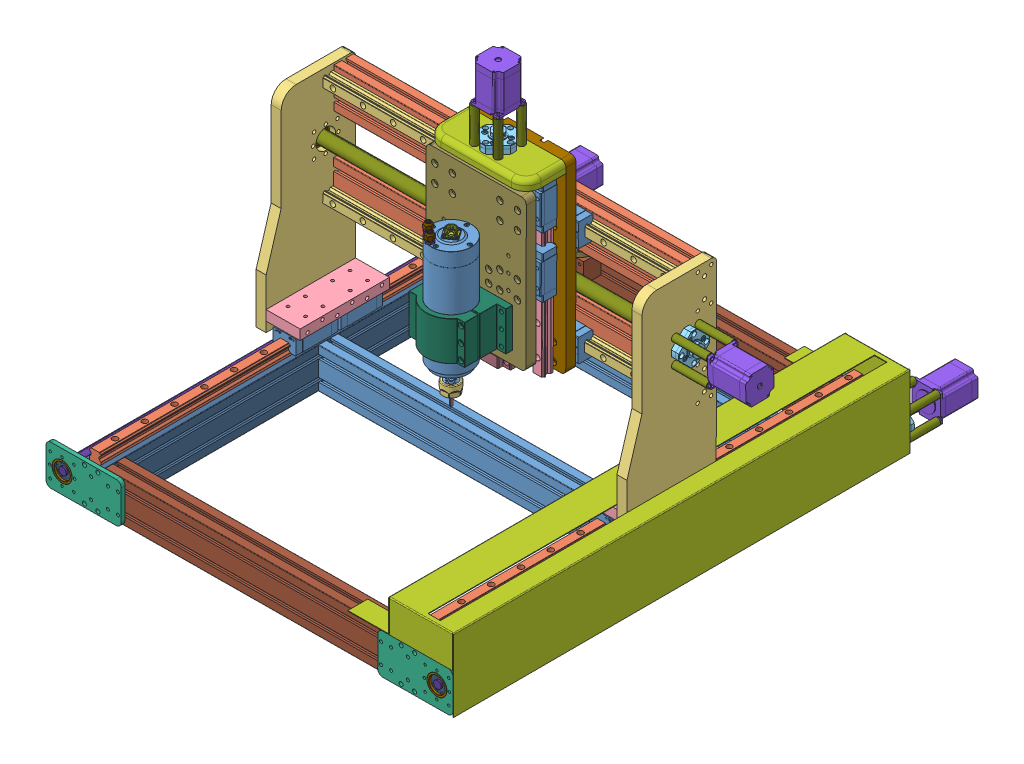
SolidWorks assembly cnc machine, configuration 默认. Lengths in mm. (continued)
Mates (geometry in assembly coordinates): (continued)
- Concentric138: concentric: cylinder of 57BYG250C-3 through (786.0531 509.1221 -21.2847) axis (-0.004945 -0.003582 -0.999981) radius 4; cylinder of FK_15Yes_FS-3/_FK_15collar_4-1 through (786.4013 509.3743 49.1139) axis (-0.004945 -0.003582 -0.999981) radius 7.5
- Parallel7: parallel: plane of back-2 through (386.56 716.0099 462.5509) normal (-0.999986 -0.00209 0.004953); plane of sfu25unit-4/slidernutSLDPRT-1 through (466.0897 826.0042 413.7627) normal (-0.999986 -0.00209 0.004953)
- Parallel8: parallel: plane of back-2 through (486.1687 901.2173 461.3948) normal (-0.004945 -0.003582 -0.999981); plane of sfu25unit-4/slidernutSLDPRT-1 through (506.0891 826.0878 413.5646) normal (-0.004945 -0.003582 -0.999981)
- Concentric178: concentric: cylinder of top plate-1 through (486.0978 1066.4165 516.8045) axis (-0.002108 0.999991 -0.003572) radius 20; cylinder of sfu25unit-5/SFU2505-1 through (486.4038 921.2727 517.3229) axis (-0.002108 0.999991 -0.003572) radius 12.5
- Parallel10: parallel: plane of back-2 through (486.2676 901.289 481.3945) normal (0.004945 0.003582 0.999981); plane of sfu25unit-5/slidernutSLDPRT-1 through (453.544 911.2898 541.5216) normal (0.004945 0.003582 0.999981)
- Concentric181: concentric: cylinder of linerrailHGGR25400-2 through (763.4076 958.1784 441.5619) axis (-0.999986 -0.00209 0.004953) radius 2.43; cylinder of HGH25CA-6 through (398.9607 957.4167 443.367) axis (0.999986 0.00209 -0.004953) radius 2.43
- Coincident354: coincident: plane of back-2 through (386.56 716.0099 462.5509) normal (-0.999986 -0.00209 0.004953); plane of motorseat-2 through (386.3277 1061.2201 561.3173) normal (-0.999986 -0.00209 0.004953)
- Coincident355: coincident: plane of back-2 through (586.5572 716.4279 461.5603) normal (0.999986 0.00209 -0.004953); plane of motorseat-2 through (586.3248 1061.6381 560.3268) normal (0.999986 0.00209 -0.004953)
- Concentric183: concentric: cylinder of linerrailHGGR25300-1 through (421.2087 981.2312 503.4303) axis (0.004945 0.003582 0.999981) radius 5.5; cylinder of back-2 through (421.001 981.0808 461.4311) axis (-0.004945 -0.003582 -0.999981) radius 2.5
- Concentric185: concentric: cylinder of HGH25CA-11 through (438.94 913.6879 521.5849) axis (0.004945 0.003582 0.999981) radius 3; cylinder of motorseat-2 through (439.1378 913.8311 561.5841) axis (0.004945 0.003582 0.999981) radius 6.5
- Concentric186: concentric: circle of top plate-1; circle of sfu25unit-5/SFU2505-1
- Concentric187: concentric: cylinder of top plate-1 through (486.0978 1066.4165 516.8045) axis (-0.002108 0.999991 -0.003572) radius 20; cylinder of sfu25unit-5/SFU2505-1 through (486.4038 921.2727 517.3229) axis (-0.002108 0.999991 -0.003572) radius 12.5
- Concentric188: concentric: cylinder of linerrailHGGR25300-1 through (432.4857 1061.2535 502.8303) axis (0.002108 -0.999991 0.003572) radius 2.43; cylinder of HGH25CA-12 through (432.5197 1045.1087 502.888) axis (0.002108 -0.999991 0.003572) radius 2.43
- Concentric189: concentric: cylinder of linerrailHGGR25300-1 through (409.5919 1061.2067 502.9437) axis (0.002108 -0.999991 0.003572) radius 2.43; cylinder of HGH25CA-12 through (409.6259 1045.0608 503.0014) axis (0.002108 -0.999991 0.003572) radius 2.43
- Concentric190: concentric: cylinder of HGH25CA-12 through (403.6876 1033.6137 521.3296) axis (0.004945 0.003582 0.999981) radius 3; cylinder of motorseat-2 through (403.8854 1033.757 561.3289) axis (0.004945 0.003582 0.999981) radius 6.5
- Coincident357: coincident: plane of HGH25CA-12 through (407.6633 1045.1219 521.2687) normal (0.004945 0.003582 0.999981); plane of 10mmwasher-1 through (422.2242 1016.1525 521.3005) normal (-0.004945 -0.003582 -0.999981)
- Coincident358: coincident: plane of HGH25CA-12 through (421.1963 987.0862 503.4094) normal (0.002108 -0.999991 0.003572); plane of 10mmwasher-1 through (447.285 987.205 521.2802) normal (0.002108 -0.999991 0.003572)
- Coincident359: coincident: plane of 10mmwasher-1 through (422.3231 1016.2241 541.3001) normal (0.004945 0.003582 0.999981); plane of motorseat-2 through (486.5435 911.3588 541.3582) normal (-0.004945 -0.003582 -0.999981)
- Concentric192: concentric: cylinder of sfu25unit-5/slidernutSLDPRT-1 through (461.5607 903.3066 541.5105) axis (0.004945 0.003582 0.999981) radius 2.5; cylinder of motorseat-2 through (461.6596 903.3782 561.5102) axis (0.004945 0.003582 0.999981) radius 3.3
- Coincident360: coincident: plane of 80_2-1 through (486.7394 865.4308 561.5221) normal (-0.004945 -0.003582 -0.999981); plane of motorseat-2 through (486.6424 911.4304 561.3578) normal (0.004945 0.003582 0.999981)
- Concentric193: concentric: cylinder of top plate-1 through (509.7433 1086.55 540.1873) axis (-0.002108 0.999991 -0.003572) radius 2.5; cylinder of motor conectors-4/motor connector-2 through (509.7433 1086.55 540.1873) axis (-0.002108 0.999991 -0.003572) radius 7
- Coincident361: coincident: plane of 57BYG250C-1 through (485.9081 1156.4157 516.483) normal (0.002108 -0.999991 0.003572); plane of motor conectors-4/motor connector-1 through (462.4536 1156.4509 540.1694) normal (-0.002108 0.999991 -0.003572)
- Concentric196: concentric: cylinder of 80_2-1 through (551.4531 796.6164 575.4488) axis (0.004945 0.003582 0.999981) radius 4; cylinder of motorseat-2 through (551.3839 796.5662 561.4491) axis (0.004945 0.003582 0.999981) radius 3.4
- Coincident363: coincident: plane of HGH25CA-12 through (397.156 1045.0946 519.8208) normal (-0.999986 -0.00209 0.004953); plane of 10mmwasher-1 through (397.1635 1045.1 521.3207) normal (-0.999986 -0.00209 0.004953)
- Concentric200: concentric: cylinder of back-2 through (513.636 726.3469 481.8858) axis (0.004945 0.003582 0.999981) radius 2.5; cylinder of BF_15-1/_BF_15_Part1_2-1 through (513.6756 726.3756 489.8856) axis (0.004945 0.003582 0.999981) radius 3.3
- Concentric201: concentric: cylinder of back-2 through (459.6368 726.234 482.1532) axis (0.004945 0.003582 0.999981) radius 2.5; cylinder of BF_15-1/_BF_15_Part1_2-1 through (459.6764 726.2627 490.1531) axis (0.004945 0.003582 0.999981) radius 5.5
- Coincident373: coincident: plane of BF_15-1/_BF_15_Part1_2-1 through (452.8554 736.2484 490.151) normal (-0.004945 -0.003582 -0.999981); plane of 8mmwasher-1 through (486.676 726.2625 490.0196) normal (0.004945 0.003582 0.999981)
- Concentric202: concentric: cylinder of BF_15-1/_BF_15_Part1_2-1 through (459.6764 726.2627 490.1531) axis (0.004945 0.003582 0.999981) radius 3.3; cylinder of 8mmwasher-1 through (459.6764 726.2627 490.1531) axis (-0.004945 -0.003582 -0.999981) radius 3
- Coincident374: coincident: plane of back-2 through (486.2676 901.289 481.3945) normal (0.004945 0.003582 0.999981); plane of 8mmwasher-1 through (486.6365 726.2338 482.0197) normal (-0.004945 -0.003582 -0.999981)
- Concentric203: concentric: cylinder of sfu25unit-5/SFU2505-1 through (486.4038 921.2727 517.3229) axis (-0.002108 0.999991 -0.003572) radius 12.5; cylinder of BF_15-1/_BF_15_Part2_4-1 through (486.7091 776.419 517.8402) axis (0.002108 -0.999991 0.003572) radius 7.5
- Concentric204: concentric: cylinder of FK_15Yes_FS-1/_FK_15_FS_1_2-1 through (800.6126 846.789 436.0343) axis (0.999986 0.00209 -0.004953) radius 6.9585; cylinder of screw2-1 through (34.6237 845.1881 439.8282) axis (-0.999986 -0.00209 0.004953) radius 12.5
- Concentric205: concentric: cylinder of FK_15Yes_FS-3/_FK_15collar_4-1 through (786.4013 509.3743 49.1139) axis (-0.004945 -0.003582 -0.999981) radius 7.5; cylinder of screw2 - right left-1 through (790.8224 512.5765 943.0973) axis (0.004945 0.003582 0.999981) radius 12.5
- Coincident376: coincident: plane of FF_15-2/_FF_15_Part2_4-1 through (789.6322 497.0249 931.1586) normal (-0.004945 -0.003582 -0.999981); plane of screw2 - right left-1 through (784.5914 523.4037 931.0891) normal (0.004945 0.003582 0.999981)
- Concentric206: concentric: cylinder of FK_15Yes_FS-2/_FK_15collar_4-1 through (38.4121 507.8109 52.8186) axis (-0.004945 -0.003582 -0.999981) radius 7.5; cylinder of screw2 - right left-2 through (42.8332 511.0132 946.8029) axis (0.004945 0.003582 0.999981) radius 12.5
- Concentric207: concentric: cylinder of FK_15Yes_FS-4/_FK_15collar_4-1 through (486.0999 1065.4165 516.8081) axis (-0.002108 0.999991 -0.003572) radius 7.5; cylinder of screw2 top-1 through (486.8387 714.9195 518.0599) axis (0.002108 -0.999991 0.003572) radius 12.5
- Concentric208: concentric: cylinder of 80_2-1 through (422.3285 856.3462 575.8734) axis (0.004945 0.003582 0.999981) radius 4; cylinder of motorseat-2 through (422.2593 856.2961 561.8737) axis (0.004945 0.003582 0.999981) radius 3.4
- Distance2: distance = 10 mm: plane of 80_2.2Kw-2/Шпиндель Ø80_2.2Kw.stp-1/D880_2.2Kw.stp-1 through (467.4776 751.469 583.8543) normal (0.002108 -0.999991 0.003572); plane of motorseat-2 through (386.96 761.2227 562.3888) normal (0.002108 -0.999991 0.003572)
- Concentric210: concentric: cylinder of linerrailHGGR25-1 through (99.5791 572.3208 719.2975) axis (-0.002108 0.999991 -0.003572) radius 5.5; cylinder of nuts-4 through (100.2578 250.3236 720.4475) axis (-0.002108 0.999991 -0.003572) radius 2.4112
- Concentric211: concentric: cylinder of linerrailHGGR25-2 through (716.7608 570.9245 36.2366) axis (0.004945 0.003582 0.999981) radius 2.43; cylinder of HGH25CA-4 through (718.9723 572.5263 483.4213) axis (0.004945 0.003582 0.999981) radius 2.43
- Coincident409: coincident: plane of bottom-1/EF4080-t5-900-2 through (712.7555 528.2383 936.4271) normal (-0.999986 -0.00209 0.004953); plane of EF4080-t5 -592-1 through (709.0064 544.7019 186.43) normal (0.999986 0.00209 -0.004953)
- Coincident410: coincident: plane of bottom-1/EF4080-t5-900-2 through (712.7046 552.3881 936.3409) normal (-0.002108 0.999991 -0.003572); plane of EF4080-t5 -592-1 through (708.897 549.6302 166.4125) normal (-0.002108 0.999991 -0.003572)
- Concentric225: concentric: cylinder of sfu25unit-3/SFU2505-1 through (788.3952 510.8185 452.2985) axis (0.004945 0.003582 0.999981) radius 12.5; cylinder of screw2 - right left-1 through (790.8224 512.5765 943.0973) axis (0.004945 0.003582 0.999981) radius 12.5
- Distance5: limit distance = 134.855 mm: plane of BF_15-1/_BF_15_Part1_2-1 through (486.7934 736.4193 517.9831) normal (-0.002108 0.999991 -0.003572); plane of sfu25unit-5/slidernutSLDPRT-1 through (506.3902 871.229 493.4029) normal (0.002108 -0.999991 0.003572)
- Concentric241: concentric: cylinder of FF_15-1/_FF_15_Part2_4-1 through (43.0434 511.1654 989.3021) axis (-0.004945 -0.003582 -0.999981) radius 7.5; cylinder of screw2 - right left-2 through (42.8332 511.0132 946.8029) axis (0.004945 0.003582 0.999981) radius 12.5
- Coincident456: coincident: plane of FK_15Yes_FS-1/_FK_15collar_4-1 through (762.6288 839.2096 436.2225) normal (-0.999986 -0.00209 0.004953); plane of screw2-1 through (762.6356 839.3453 437.6426) normal (0.999986 0.00209 -0.004953)
- Coincident457: coincident: plane of FF_15-1/_FF_15_Part2_4-1 through (42.6559 495.4208 934.8594) normal (-0.004945 -0.003582 -0.999981); plane of screw2 - right left-2 through (38.9401 499.0728 934.8647) normal (0.004945 0.003582 0.999981)
- Coincident458: coincident: plane of 57BYG250C-2 through (37.9621 507.485 -38.1797) normal (0.004945 0.003582 0.999981); plane of motor conectors-5/motor connector-1 through (14.3427 531.0055 -38.1471) normal (-0.004945 -0.003582 -0.999981)
- Coincident459: coincident: plane of BF_15-1/_BF_15_Part2_4-1 through (486.7664 730.8914 510.2029) normal (-0.002108 0.999991 -0.003572); plane of screw2 top-1 through (474.3221 730.8954 518.657) normal (0.002108 -0.999991 0.003572)
- Coincident462: coincident: plane of linerrailHGGR25-1 through (112.2132 551.133 939.315) normal (0.002108 -0.999991 0.003572); plane of bottom-1/EF4080-t5-900-1 through (120.7131 551.1508 939.2729) normal (-0.002108 0.999991 -0.003572)
- Coincident463: coincident: plane of nuts-4 through (93.4719 547.0939 939.4222) normal (-0.002108 0.999991 -0.003572); plane of bottom-1/EF4080-t5-900-1 through (96.5719 547.1004 939.4068) normal (0.002108 -0.999991 0.003572)
- Coincident464: coincident: plane of nuts-4 through (96.5719 547.1004 939.4068) normal (-0.999986 -0.00209 0.004953); plane of bottom-1/EF4080-t5-900-1 through (96.5635 551.1003 939.3925) normal (0.999986 0.00209 -0.004953)
- Concentric252: concentric: cylinder of linerrailHGGR25-1 through (99.8758 572.5357 779.2964) axis (-0.002108 0.999991 -0.003572) radius 5.5; cylinder of nuts-4 through (100.5545 250.5385 780.4464) axis (-0.002108 0.999991 -0.003572) radius 2.4112
- Coincident469: coincident: plane of side right - final-5 through (64.7984 569.6809 560.668) normal (0.004945 0.003582 0.999981); plane of bottom-2 through (132.7131 609.8227 560.1884) normal (0.004945 0.003582 0.999981)
- Coincident473: coincident: plane of HGH25CA-2 through (120.4444 589.2114 396.3198) normal (-0.002108 0.999991 -0.003572); plane of bottom-2 through (98.3107 589.4294 470.4299) normal (0.002108 -0.999991 0.003572)
- Coincident477: coincident: plane of sfu25unit-1/slidernutSLDPRT-1 through (64.0888 542.1259 405.7674) normal (0.999986 0.00209 -0.004953); plane of conn12-1 through (63.8661 589.036 380.6) normal (-0.999986 -0.00209 0.004953)
- Concentric257: concentric: cylinder of sfu25unit-1/SFU2505-1 through (40.1093 509.0402 396.0043) axis (-0.004945 -0.003582 -0.999981) radius 12.5; cylinder of FK_15Yes_FS-2/_FK_15_FS_1_2-1 through (38.3923 507.7966 48.8187) axis (-0.004945 -0.003582 -0.999981) radius 20
- Concentric259: concentric: cylinder of 57BYG250C-2 through (14.3427 531.0055 -38.1471) axis (-0.004945 -0.003582 -0.999981) radius 2.55; cylinder of motor conectors-5/motor connector-1 through (14.3427 531.0055 -38.1471) axis (0.004945 0.003582 0.999981) radius 3
- Concentric260: concentric: cylinder of FK_15Yes_FS-2/_FK_15_FS_1_2-1 through (38.3923 507.7966 48.8187) axis (-0.004945 -0.003582 -0.999981) radius 20; cylinder of mot1-1 through (38.3082 507.7357 31.819) axis (0.004945 0.003582 0.999981) radius 20
- Concentric261: concentric: cylinder of bottom-1/EF4080-t5-900-1 through (87.2273 544.5808 939.462) axis (-0.004945 -0.003582 -0.999981) radius 4; cylinder of mot1-1 through (82.7765 541.3571 39.4788) axis (0.004945 0.003582 0.999981) radius 4
- Concentric262: concentric: cylinder of bottom-1/EF4080-t5-900-1 through (114.2269 544.6373 939.3283) axis (-0.004945 -0.003582 -0.999981) radius 4; circle of mot1-1
- Coincident483: coincident: plane of bottom-1/EF4080-t5-900-1 through (96.4207 472.8859 39.6566) normal (-0.004945 -0.003582 -0.999981); plane of mot1-1 through (81.3472 507.8542 39.6059) normal (0.004945 0.003582 0.999981)
- Coincident484: coincident: plane of FK_15Yes_FS-2/_FK_15_FS_1_2-1 through (38.2429 538.7354 31.7083) normal (0.004945 0.003582 0.999981); plane of mot1-1 through (81.3076 507.8256 31.6061) normal (-0.004945 -0.003582 -0.999981)
- Concentric263: concentric: cylinder of FK_15Yes_FS-2/_FK_15_FS_1_2-1 through (38.2555 532.7355 31.7297) axis (-0.004945 -0.003582 -0.999981) radius 4.75; cylinder of mot1-1 through (38.2951 532.7641 39.7296) axis (0.004945 0.003582 0.999981) radius 2.5
- Concentric264: concentric: cylinder of motor conectors-5/motor connector-1 through (14.3427 531.0055 -38.1471) axis (0.004945 0.003582 0.999981) radius 7; cylinder of mot1-1 through (14.7285 531.2849 39.8514) axis (0.004945 0.003582 0.999981) radius 2.5
- Parallel11: parallel: plane of 57BYG250C-2 through (21.3864 535.4216 -102.199) normal (-0.002108 0.999991 -0.003572); plane of mot1-1 through (6.2639 547.6971 39.8345) normal (-0.002108 0.999991 -0.003572)
- Coincident485: coincident: plane of motor conectors-5/motor connector-1 through (14.6889 531.2562 31.8516) normal (0.004945 0.003582 0.999981); plane of mot1-1 through (81.3076 507.8256 31.6061) normal (-0.004945 -0.003582 -0.999981)
- Coincident486: coincident: plane of linerrailHGGR25-1 through (96.2163 569.8851 39.3102) normal (-0.004945 -0.003582 -0.999981); plane of bottom-1/EF4080-t5 -540-2 through (708.2538 549.1643 36.3576) normal (-0.004945 -0.003582 -0.999981)
- Concentric266: concentric: cylinder of linerrailHGGR25-2 through (716.7608 570.9245 36.2366) axis (0.004945 0.003582 0.999981) radius 2.43; cylinder of HGH25CA-3 through (718.5272 572.204 393.423) axis (0.004945 0.003582 0.999981) radius 2.43
- Coincident487: coincident: plane of linerrailHGGR25-2 through (744.2041 552.4539 936.1848) normal (0.002108 -0.999991 0.003572); plane of bottom-1/EF4080-t5-900-2 through (752.704 552.4717 936.1427) normal (-0.002108 0.999991 -0.003572)
- Concentric268: concentric: cylinder of EF4080-t5 -800-1 through (763.2626 960.1301 413.3126) axis (-0.999986 -0.00209 0.004953) radius 4; cylinder of side right - final-5 through (63.2728 958.6671 416.7796) axis (0.999986 0.00209 -0.004953) radius 3.4
- Concentric269: concentric: cylinder of EF4080-t5 -800-1 through (763.4039 893.1307 413.5519) axis (-0.999986 -0.00209 0.004953) radius 4; cylinder of side right - final-5 through (63.414 891.6677 417.0189) axis (0.999986 0.00209 -0.004953) radius 3.4
- Coincident488: coincident: plane of EF4080-t5 -800-1 through (63.3504 890.1194 403.5245) normal (-0.999986 -0.00209 0.004953); plane of side right - final-5 through (63.7314 789.1454 437.8425) normal (0.999986 0.00209 -0.004953)
- Concentric271: concentric: cylinder of EF4080-t5 -800-2 through (763.5999 800.1315 413.8841) axis (-0.999986 -0.00209 0.004953) radius 4; cylinder of side right - final-5 through (63.61 798.6685 417.351) axis (0.999986 0.00209 -0.004953) radius 3.4
- Concentric272: concentric: cylinder of EF4080-t5 -800-1 through (763.1291 960.0334 386.3131) axis (-0.999986 -0.00209 0.004953) radius 4; cylinder of side right - final-6 through (783.1288 960.0752 386.2141) axis (0.999986 0.00209 -0.004953) radius 3.4
- Coincident489: coincident: plane of EF4080-t5 -800-2 through (763.6775 731.5837 400.629) normal (0.999986 0.00209 -0.004953); plane of side right - final-6 through (763.7213 790.6084 434.3756) normal (-0.999986 -0.00209 0.004953)
- Concentric273: concentric: cylinder of EF4080-t5 -800-2 through (763.6076 733.0354 387.1239) axis (-0.999986 -0.00209 0.004953) radius 4; cylinder of side right - final-6 through (783.6073 733.0772 387.0248) axis (0.999986 0.00209 -0.004953) radius 3.4
- Coincident490: coincident: plane of EF4080-t5 -800-2 through (63.6876 730.1207 404.0959) normal (-0.999986 -0.00209 0.004953); plane of side right - final-5 through (63.7314 789.1454 437.8425) normal (0.999986 0.00209 -0.004953)
- Coincident493: coincident: plane of nuts-3 through (737.7867 546.869 496.2284) normal (-0.002108 0.999991 -0.003572); plane of bottom-1/EF4080-t5-900-2 through (736.8626 548.4386 936.2355) normal (0.002108 -0.999991 0.003572)
- Coincident494: coincident: plane of nuts-3 through (726.3784 550.8452 496.2706) normal (-0.999986 -0.00209 0.004953); plane of bottom-1/EF4080-t5-900-2 through (728.5543 552.4212 936.2624) normal (0.999986 0.00209 -0.004953)
- Concentric276: concentric: cylinder of linerrailHGGR25-2 through (730.6798 572.9969 536.1707) axis (-0.002108 0.999991 -0.003572) radius 5.5; cylinder of nuts-3 through (731.3585 250.9997 537.3207) axis (-0.002108 0.999991 -0.003572) radius 2.4112
- Concentric277: concentric: cylinder of linerrailHGGR25-2 through (731.2732 573.4268 656.1684) axis (-0.002108 0.999991 -0.003572) radius 3.5; cylinder of nuts-3 through (731.9519 251.4295 657.3185) axis (-0.002108 0.999991 -0.003572) radius 2.4112
- Concentric278: concentric: cylinder of HGH25CA-1 through (116.1195 589.6899 532.8421) axis (-0.002108 0.999991 -0.003572) radius 3; cylinder of bottom-2 through (116.0774 609.6897 532.7706) axis (-0.002108 0.999991 -0.003572) radius 3
- Coincident496: coincident: plane of side right - final-5 through (63.7314 789.1454 437.8425) normal (0.999986 0.00209 -0.004953); plane of bottom-2 through (64.7141 609.6806 560.5252) normal (-0.999986 -0.00209 0.004953)
- Concentric279: concentric: cylinder of side right - final-5 through (64.6694 595.6269 545.5755) axis (0.999986 0.00209 -0.004953) radius 4; cylinder of bottom-2 through (64.6694 595.6269 545.5755) axis (-0.999986 -0.00209 0.004953) radius 3.4
- Concentric280: concentric: cylinder of side right - final-5 through (63.9529 583.0898 395.6211) axis (0.999986 0.00209 -0.004953) radius 4; cylinder of conn12-1 through (63.9529 583.0898 395.6211) axis (-0.999986 -0.00209 0.004953) radius 3.4
- Concentric281: concentric: cylinder of side right - final-5 through (64.2497 583.3047 455.62) axis (0.999986 0.00209 -0.004953) radius 4; cylinder of conn12-1 through (64.2497 583.3047 455.62) axis (-0.999986 -0.00209 0.004953) radius 3.4
- Concentric282: concentric: cylinder of HGH25CA-2 through (80.5019 589.169 408.0177) axis (-0.002108 0.999991 -0.003572) radius 3; cylinder of bottom-2 through (80.4597 609.1688 407.9463) axis (-0.002108 0.999991 -0.003572) radius 3
- Coincident498: coincident: plane of linerrailHGGR25400-3 through (763.8536 746.7341 442.5746) normal (0.999986 0.00209 -0.004953); plane of side right - final-6 through (763.7213 790.6084 434.3756) normal (-0.999986 -0.00209 0.004953)
- Concentric285: concentric: cylinder of side right - final-6 through (783.9004 604.5944 391.9837) axis (0.999986 0.00209 -0.004953) radius 4; cylinder of bottom-3 through (695.9017 604.4105 392.4195) axis (-0.999986 -0.00209 0.004953) radius 3.4
- Coincident502: coincident: plane of side right - final-6 through (763.7213 790.6084 434.3756) normal (-0.999986 -0.00209 0.004953); plane of bottom-3 through (763.856 590.499 377.133) normal (0.999986 0.00209 -0.004953)
- Concentric286: concentric: cylinder of side right - final-6 through (784.659 597.1318 542.0094) axis (0.999986 0.00209 -0.004953) radius 4; cylinder of bottom-3 through (696.6603 596.9478 542.4453) axis (-0.999986 -0.00209 0.004953) radius 3.4
- Coincident503: coincident: plane of side right - final-6 through (763.7213 790.6084 434.3756) normal (-0.999986 -0.00209 0.004953); plane of conn12-2 through (764.3011 590.8214 467.1313) normal (0.999986 0.00209 -0.004953)
- Concentric288: concentric: cylinder of side right - final-6 through (783.9425 584.5946 392.0551) axis (0.999986 0.00209 -0.004953) radius 4; cylinder of conn12-2 through (763.9428 584.5528 392.1542) axis (0.999986 0.00209 -0.004953) radius 3.4
- Concentric289: concentric: cylinder of side right - final-6 through (784.2393 584.8095 452.054) axis (0.999986 0.00209 -0.004953) radius 4; cylinder of conn12-2 through (764.2396 584.7677 452.153) axis (0.999986 0.00209 -0.004953) radius 3.4
- Concentric290: concentric: cylinder of sfu25unit-3/slidernutSLDPRT-1 through (764.2538 535.7036 434.3284) axis (-0.999986 -0.00209 0.004953) radius 2.5; cylinder of conn12-2 through (764.2538 535.7036 434.3284) axis (0.999986 0.00209 -0.004953) radius 6.5
- Concentric291: concentric: cylinder of sfu25unit-3/slidernutSLDPRT-1 through (764.1351 535.6177 410.3288) axis (-0.999986 -0.00209 0.004953) radius 2.5; cylinder of conn12-2 through (764.1351 535.6177 410.3288) axis (0.999986 0.00209 -0.004953) radius 6.5
- Coincident504: coincident: plane of sfu25unit-3/slidernutSLDPRT-1 through (764.2765 543.7322 442.2997) normal (-0.999986 -0.00209 0.004953); plane of conn12-2 through (764.3011 590.8214 467.1313) normal (0.999986 0.00209 -0.004953)
- Concentric292: concentric: cylinder of bottom-1/EF4080-t5-900-2 through (719.2182 545.9017 936.3319) axis (-0.004945 -0.003582 -0.999981) radius 4; cylinder of mot1-2 through (714.7674 542.678 36.3487) axis (0.004945 0.003582 0.999981) radius 4
- Coincident505: coincident: plane of bottom-1/EF4080-t5-900-2 through (728.2641 544.2062 36.2764) normal (-0.004945 -0.003582 -0.999981); plane of mot1-2 through (743.3376 509.2378 36.3272) normal (0.004945 0.003582 0.999981)
- Concentric293: concentric: cylinder of FK_15Yes_FS-3/_FK_15_FS_1_2-1 through (786.3815 509.3599 45.114) axis (-0.004945 -0.003582 -0.999981) radius 20; cylinder of mot1-2 through (786.2974 509.2991 28.1143) axis (0.004945 0.003582 0.999981) radius 20
- Coincident506: coincident: plane of FK_15Yes_FS-3/_FK_15_FS_1_2-1 through (786.2298 540.2988 28.0036) normal (0.004945 0.003582 0.999981); plane of mot1-2 through (743.298 509.2092 28.3273) normal (-0.004945 -0.003582 -0.999981)
- Concentric294: concentric: cylinder of HGH25CA-4 through (713.1109 590.9376 529.8852) axis (-0.002108 0.999991 -0.003572) radius 3; cylinder of bottom-3 through (713.1109 590.9376 529.8852) axis (0.002108 -0.999991 0.003572) radius 3
- Concentric295: concentric: cylinder of HGH25CA-3 through (712.4927 590.4899 404.8876) axis (-0.002108 0.999991 -0.003572) radius 3; cylinder of bottom-3 through (712.4927 590.4899 404.8876) axis (0.002108 -0.999991 0.003572) radius 3
- Coincident507: coincident: plane of linerrailHGGR25-2 through (728.2071 571.206 36.18) normal (-0.004945 -0.003582 -0.999981); plane of mot1-2 through (743.3376 509.2378 36.3272) normal (0.004945 0.003582 0.999981)
- Coincident508: coincident: plane of motor conectors-1/motor connector-1 through (760.9197 533.2118 28.1542) normal (0.004945 0.003582 0.999981); plane of mot1-2 through (743.298 509.2092 28.3273) normal (-0.004945 -0.003582 -0.999981)
- Coincident509: coincident: plane of bottom-1/EF4080-t5-900-1 through (100.8715 476.1097 939.6398) normal (0.004945 0.003582 0.999981); plane of mot1-4 through (85.7979 511.078 939.5891) normal (-0.004945 -0.003582 -0.999981)
- Concentric296: concentric: cylinder of bottom-1/EF4080-t5-900-1 through (114.2269 544.6373 939.3283) axis (-0.004945 -0.003582 -0.999981) radius 4; cylinder of mot1-4 through (114.2665 544.6659 947.3282) axis (0.004945 0.003582 0.999981) radius 4
- Concentric297: concentric: circle of sfu25unit-1/slidernutSLDPRT-1; cylinder of conn12-1 through (64.2639 534.2406 437.7953) axis (-0.999986 -0.00209 0.004953) radius 6.5
- Coincident510: coincident: plane of FF_15-2/_FF_15Part1_2-1 through (793.0421 543.4692 935.9755) normal (0.004945 0.003582 0.999981); plane of mot1-3 through (747.7884 512.4616 936.3104) normal (-0.004945 -0.003582 -0.999981)
- Concentric298: concentric: cylinder of FF_15-2/_FF_15Part1_2-1 through (790.5405 512.3724 886.0983) axis (0.004945 0.003582 0.999981) radius 20; cylinder of mot1-3 through (790.7877 512.5515 936.0974) axis (0.004945 0.003582 0.999981) radius 20
- Concentric299: concentric: cylinder of FF_15-2/_FF_15_Part2_4-1 through (791.0325 512.7288 985.5965) axis (-0.004945 -0.003582 -0.999981) radius 7.5; cylinder of screw2 - right left-1 through (790.8224 512.5765 943.0973) axis (0.004945 0.003582 0.999981) radius 12.5
- Coincident511: coincident: plane of bottom-1/EF4080-t5-900-2 through (732.7148 547.4299 936.2597) normal (0.004945 0.003582 0.999981); plane of mot1-3 through (747.7884 512.4616 936.3104) normal (-0.004945 -0.003582 -0.999981)
- Concentric300: concentric: cylinder of bottom-1/EF4080-t5-900-2 through (719.2182 545.9017 936.3319) axis (-0.004945 -0.003582 -0.999981) radius 4; cylinder of mot1-3 through (719.2577 545.9304 944.3317) axis (0.004945 0.003582 0.999981) radius 4
- Coincident512: coincident: plane of linerrailHGGR25400-2 through (63.3576 933.6906 423.3687) normal (-0.004945 -0.003582 -0.999981); plane of EF4080-t5 -800-1 through (763.3988 910.8038 419.9887) normal (0.004945 0.003582 0.999981)
- Concentric304: concentric: cylinder of screw2-1 through (34.6237 845.1881 439.8282) axis (-0.999986 -0.00209 0.004953) radius 12.5; cylinder of side right - final-6 through (763.6131 846.7117 436.2176) axis (0.999986 0.00209 -0.004953) radius 20
- Coincident513: coincident: plane of FK_15Yes_FS-1/_FK_15_FS_1_2-1 through (783.6776 815.7536 436.1184) normal (-0.999986 -0.00209 0.004953); plane of side right - final-6 through (783.721 790.6502 434.2765) normal (0.999986 0.00209 -0.004953)
- Concentric305: concentric: cylinder of motor conectors-3/motor connector-4 through (783.4466 870.2389 412.4648) axis (0.999986 0.00209 -0.004953) radius 7; cylinder of side right - final-6 through (783.4466 870.2389 412.4648) axis (0.999986 0.00209 -0.004953) radius 3.4
- Coincident514: coincident: plane of motor conectors-3/motor connector-4 through (783.4466 870.2389 412.4648) normal (-0.999986 -0.00209 0.004953); plane of side right - final-6 through (783.721 790.6502 434.2765) normal (0.999986 0.00209 -0.004953)
- Concentric306: concentric: cylinder of FF_15-3/_FF_15Part1_2-1 through (-6.3757 845.1024 440.0312) axis (0.999986 0.00209 -0.004953) radius 20; cylinder of side right - final-5 through (43.6235 845.2069 439.7836) axis (0.999986 0.00209 -0.004953) radius 20
- Coincident515: coincident: plane of FF_15-3/_FF_15Part1_2-1 through (43.7747 846.3025 470.7638) normal (0.999986 0.00209 -0.004953); plane of side right - final-5 through (43.7317 789.1036 437.9416) normal (-0.999986 -0.00209 0.004953)
- Concentric307: concentric: cylinder of sfu25unit-4/SFU2505-1 through (516.1655 846.1945 437.4431) axis (0.999986 0.00209 -0.004953) radius 12.5; cylinder of screw2-1 through (34.6237 845.1881 439.8282) axis (-0.999986 -0.00209 0.004953) radius 12.5
- Coincident516: coincident: plane of nuts-2 through (463.2925 953.2621 417.3207) normal (0.004945 0.003582 0.999981); plane of EF4080-t5 -800-1 through (763.2947 950.7892 415.846) normal (-0.004945 -0.003582 -0.999981)
- Coincident517: coincident: plane of nuts-2 through (463.3231 938.7623 417.3725) normal (0.002108 -0.999991 0.003572); plane of EF4080-t5 -800-1 through (763.3187 939.3893 415.8867) normal (-0.002108 0.999991 -0.003572)
- Coincident518: coincident: plane of nuts-1 through (723.7168 750.7073 416.7584) normal (0.004945 0.003582 0.999981); plane of EF4080-t5 -800-2 through (763.7163 750.7909 416.5603) normal (-0.004945 -0.003582 -0.999981)
- Coincident519: coincident: plane of nuts-1 through (723.7103 753.8073 416.7473) normal (-0.002108 0.999991 -0.003572); plane of EF4080-t5 -800-2 through (763.7097 753.8909 416.5492) normal (0.002108 -0.999991 0.003572)
- Concentric308: concentric: cylinder of back-2 through (474.331 871.2641 481.5611) axis (0.004945 0.003582 0.999981) radius 3.3; cylinder of sfu25unit-4/slidernutSLDPRT-1 through (474.2321 871.1925 461.5614) axis (0.004945 0.003582 0.999981) radius 2.5
- Coincident520: coincident: plane of mot1-4 through (10.7543 550.9496 947.8176) normal (-0.999986 -0.00209 0.004953); plane of track cover-1 through (8.3414 614.7963 487.5922) normal (0.999986 0.00209 -0.004953)
- Concentric309: concentric: cylinder of bottom-1/EF4080-t5-900-1 through (87.2273 544.5808 939.462) axis (-0.004945 -0.003582 -0.999981) radius 4; cylinder of mot1-4 through (87.2669 544.6095 947.4619) axis (0.004945 0.003582 0.999981) radius 4
- Coincident522: coincident: plane of mot1-3 through (822.9112 472.6474 944.0816) normal (0.999986 0.00209 -0.004953); plane of track cover-2 through (820.3332 614.7984 483.5766) normal (-0.999986 -0.00209 0.004953)
- Coincident523: coincident: plane of mot1-3 through (747.8279 512.4903 944.3102) normal (0.004945 0.003582 0.999981); plane of track cover-2 through (758.809 616.3128 943.884) normal (0.004945 0.003582 0.999981)
- Coincident524: coincident: plane of bottom-1/EF4080-t5 -540-1 through (120.7131 551.1508 939.2729) normal (-0.002108 0.999991 -0.003572); plane of track cover-2 through (756.6686 550.8656 484.1205) normal (0.002108 -0.999991 0.003572)
